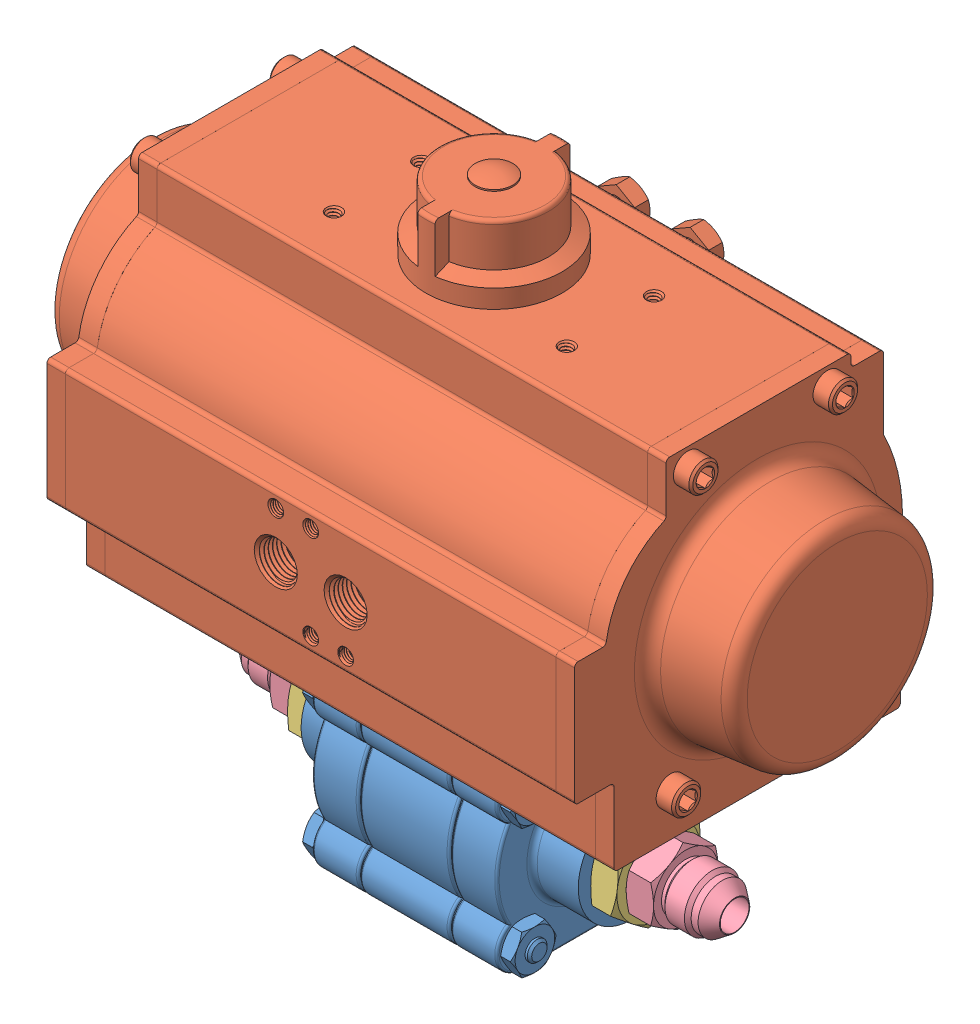
SolidWorks assembly FAKE_SOV-1,2,5, configuration Default. Lengths in mm.
Overall size (235.97 211.39 123.09).
6 component instances, 4 part files, 8 mates.
Components (placement in the parent):
- FAKE_sharpe_80BV-1: FAKE_sharpe_80BV [3778T941] at origin size (96.68 86.36 61.47)
- 49935K880_AIR ACTUATOR FOR BALL-BUTTERFLY VALVE-1: 49935K880_AIR ACTUATOR FOR BALL-BUTTERFLY VALVE [49935K88] at (0 41.529 0) x (0 0 1) z (-1 0 0) size (123.09 139.45 235.97)
- 51205K359_EXTREME-PRESSURE 316 SS THREADED PIPE FITTING-1: 51205K359_EXTREME-PRESSURE 316 SS THREADED PIPE FITTING [51205K359] at (-41.6814 0 0) x (-1 0 0) z (0 -0.924225 -0.381849) size (30.4 33 28.57)
- 50715K802-1: 50715K802 [50715K802] at (-60.0964 0 0) x (-1 0 0) z (0 0 -1) size (55.21 25.66 22.23)
- 50715K802-2: 50715K802 [50715K802] at (60.0964 0 0) size (55.21 25.66 22.23)
- 51205K359_EXTREME-PRESSURE 316 SS THREADED PIPE FITTING-3: 51205K359_EXTREME-PRESSURE 316 SS THREADED PIPE FITTING [51205K359] at (41.6814 0 0) x (1 0 0) z (0 -0.924225 -0.381849) size (30.4 33 28.57)
Mates (geometry in assembly coordinates):
- Distance1: distance = 3.175 mm anti-aligned: plane of FAKE_sharpe_80BV-1 through (0 38.354 0) normal (0 1 0); plane of 49935K880_AIR ACTUATOR FOR BALL-BUTTERFLY VALVE-1 through (-90.6462 41.529 -49.022) normal (0 -1 0)
- Concentric1: concentric anti-aligned: circle of FAKE_sharpe_80BV-1; circle of 49935K880_AIR ACTUATOR FOR BALL-BUTTERFLY VALVE-1
- Parallel1: parallel aligned: line of FAKE_sharpe_80BV-1 through (-31.75 -29.972 -22.225) axis (0 0 1); line of 49935K880_AIR ACTUATOR FOR BALL-BUTTERFLY VALVE-1 through (-90.6462 41.529 -47.752) axis (0 0 1)
- Concentric2: concentric anti-aligned: cylinder of FAKE_sharpe_80BV-1 through (-31.75 0 0) axis (-1 0 0) radius 18.669; cone of 51205K359_EXTREME-PRESSURE 316 SS THREADED PIPE FITTING-1 through (-26.8224 0 0) axis (1 0 0)
- Coincident1: coincident anti-aligned: plane of FAKE_sharpe_80BV-1 through (-47.625 0 0) normal (-1 0 0); plane of 51205K359_EXTREME-PRESSURE 316 SS THREADED PIPE FITTING-1 through (-47.625 -3.7554 -28.3272) normal (1 0 0)
- Concentric3: concentric anti-aligned: cylinder of FAKE_sharpe_80BV-1 through (-31.75 0 0) axis (-1 0 0) radius 18.669; cone of 0500_OD_JIC_to_0500_NPT-1 through (-56.5404 0 0) axis (1 0 0)
- Coincident2: coincident anti-aligned: plane of 51205K359_EXTREME-PRESSURE 316 SS THREADED PIPE FITTING-1 through (-56.5404 -3.7554 -28.3272) normal (-1 0 0); plane of 0500_OD_JIC_to_0500_NPT-1 through (-56.5404 -2.9208 -22.0322) normal (1 0 0)
- Parallel2: parallel aligned: plane of 50715K802-1 through (-60.0964 0 0) normal (0 1 0)
